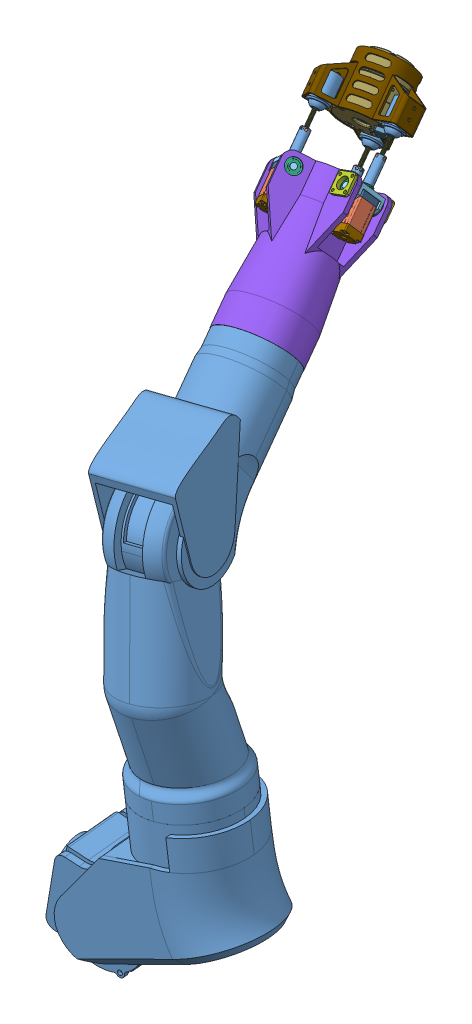
SolidWorks assembly 渲染用胳膊, configuration 默认. Lengths in mm.
Overall size (269.63 745.23 465.89).
177 component instances, 62 part files, 2 mates.
Components (placement in the parent):
- 左臂1-1: 左臂1 [默认] at (-529.8701 -324.4929 522.6027) size (209.74 530.01 223.26)
- 机械臂总装-1: 机械臂总装 [默认] at (59.2717 406.9847 293.0441) x (0.966024 0.189112 -0.176168) z (0.050994 0.528759 0.847239) size (122.17 276.98 210.32)
  - CRA-RI40-52-PRO-XX 2023.5.4 - Drum-1: CRA-RI40-52-PRO-XX 2023.5.4 - Drum [默认] at (-65.3352 0.778 -52.4868) x (-0.773511 0.267701 0.574471) z (-0.632199 -0.261859 -0.729215) size (67.95 60.31 67.96)
    - CRA-RI40-52-PRO-XX 2023.5.4 - Drum.stp-1: CRA-RI40-52-PRO-XX 2023.5.4 - Drum.stp [默认] at origin size (67.95 60.31 67.96)
      - CRA-RI40-52-PRO-XX_1_ASM.stp-1: CRA-RI40-52-PRO-XX_1_ASM.stp [默认] at origin size (67.95 60.31 67.96)
        - XB11-52__10001_ASM.stp-1: XB11-52__10001_ASM.stp [默认] at (0 16.8 0) x (0.703875 0 -0.710324) z (-0.710324 0 -0.703875) size (66.32 0.8 66.32)
          - XB11-52-06__10001.stp-1: XB11-52-06__10001.stp [默认] at (0 15.8 0) x (0.791272 0 -0.611464) z (-0.611464 0 -0.791272) size (47.28 0.81 47.28)
        - TINYMBS20WITHCONNECTOR2_ASM.stp-1: TINYMBS20WITHCONNECTOR2_ASM.stp [默认] at (2.7275 -27.9719 -6.5848) x (0 -1 0) z (0.92388 0 0.382683) size (0.82 3.25 5.53)
          - FH34SRJ8S05SH_STEP_STEP_ASM.stp-1: FH34SRJ8S05SH_STEP_STEP_ASM.stp [默认] at (-6.4719 -22.2833 0) x (0 0 -1) z (1 0 0) size (5.53 3.25 0.82)
            - NONE-51348.stp-1: NONE-51348.stp [默认] at origin size (0.15 0.3 0.08)
            - NONE-53783.stp-1: NONE-53783.stp [默认] at origin size (0.15 0.3 0.08)
            - NONE-55744.stp-1: NONE-55744.stp [默认] at origin size (0.15 0.08 0.08)
            - NONE-57763.stp-1: NONE-57763.stp [默认] at origin size (0.15 0.08 0.08)
            - NONE-60582.stp-1: NONE-60582.stp [默认] at origin size (0.15 0.3 0.08)
            - NONE-60979.stp-1: NONE-60979.stp [默认] at origin size (0.15 0.3 0.08)
            - NONE-62950.stp-1: NONE-62950.stp [默认] at origin size (0.15 0.3 0.08)
            - NONE-64179.stp-1: NONE-64179.stp [默认] at origin size (0.15 0.3 0.08)
            - NONE-65774.stp-1: NONE-65774.stp [默认] at origin size (0.15 0.08 0.08)
            - NONE-66548.stp-1: NONE-66548.stp [默认] at origin size (0.15 0.35 0.23)
            - NONE-67775.stp-1: NONE-67775.stp [默认] at origin size (0.15 0.35 0.23)
            - NONE-133224.stp-1: NONE-133224.stp [默认] at origin size (0.15 0.08 0.08)
            - NONE-134873.stp-1: NONE-134873.stp [默认] at origin size (0.15 0.3 0.08)
            - NONE-136443.stp-1: NONE-136443.stp [默认] at origin size (0.15 0.08 0.08)
            - NONE-141250.stp-1: NONE-141250.stp [默认] at origin size (0.15 0.35 0.23)
            - NONE-145287.stp-1: NONE-145287.stp [默认] at origin size (0.15 0.08 0.08)
            - NONE-147294.stp-1: NONE-147294.stp [默认] at origin size (0.15 0.08 0.08)
            - NONE-214429.stp-1: NONE-214429.stp [默认] at origin size (0.15 0.9 0.82)
            - NONE-214822.stp-1: NONE-214822.stp [默认] at origin size (0.15 0.3 0.08)
            - NONE-215190.stp-1: NONE-215190.stp [默认] at origin size (0.15 0.08 0.08)
            - NONE-216041.stp-1: NONE-216041.stp [默认] at origin size (0.15 0.35 0.23)
            - NONE-217624.stp-1: NONE-217624.stp [默认] at origin size (0.15 0.35 0.23)
            - NONE-222885.stp-1: NONE-222885.stp [默认] at origin size (0.15 0.35 0.23)
            - NONE-224875.stp-1: NONE-224875.stp [默认] at origin size (0.15 0.35 0.23)
            - NONE-228113.stp-1: NONE-228113.stp [默认] at origin size (0.15 0.9 0.82)
            - NONE-228916.stp-1: NONE-228916.stp [默认] at origin size (0.15 0.35 0.23)
        - CROSS_RECESSED_COUNTERSUNK_HE_1.stp-1: CROSS_RECESSED_COUNTERSUNK_HE_1.stp [默认] at (-21.8123 -33.1 2.8703) x (0 1 0) z (0.6 0 0.8) size (4 3.5 3.5)
        - RI40-52-D12-02__1000.stp-1: RI40-52-D12-02__1000.stp [默认] at (0 -15 0) x (0.382683 0 -0.92388) z (0.92388 0 0.382683) size (52.01 56.6 52)
        - CROSS_RECESSED_CHEESE_HEAD_SC_1.stp-1: CROSS_RECESSED_CHEESE_HEAD_SC_1.stp [默认] at (3.9505 15.5 -22.4044) x (0 -1 0) z (1 0 0) size (5.7 2.98 2.98)
        - MC50-D25X12_5_000.stp-1: MC50-D25X12_5_000.stp [默认] at (0.0001 -26.6014 0.0001) x (0.382686 0 -0.923879) z (0 -1 0) size (48.11 50.01 13.43)
        - CROSS_RECESSED_CHEESE_HEAD_SC_1.stp-2: CROSS_RECESSED_CHEESE_HEAD_SC_1.stp [默认] at (-3.9505 15.5 22.4044) x (0 -1 0) z (-1 0 0) size (5.7 2.98 2.98)
        - CROSS_RECESSED_COUNTERSUNK_HE_1.stp-2: CROSS_RECESSED_COUNTERSUNK_HE_1.stp [默认] at (-3.0048 -33.1 22.5417) x (0 1 0) z (0.395734 0 0.918365) size (4 3.5 3.5)
        - CROSS_RECESSED_CHEESE_HEAD_SC_1.stp-3: CROSS_RECESSED_CHEESE_HEAD_SC_1.stp [默认] at (-18.6357 15.5 13.0489) x (0 -1 0) z (-0.707107 0 -0.707107) size (5.7 2.98 2.98)
        - CROSS_RECESSED_COUNTERSUNK_HE_1.stp-3: CROSS_RECESSED_COUNTERSUNK_HE_1.stp [默认] at (18.8645 -33.1 -12.4259) x (0 1 0) z (0.188455 0 0.982082) size (4 3.5 3.5)
        - _M2X3_M2X3_100.stp-1: _M2X3_M2X3_100.stp [默认] at (-21.8118 -29.6014 2.8705) x (0.8 0 -0.6) z (0.6 0 0.8) size (3.23 5.8 2.8)
        - _M2X3_M2X3_100.stp-2: _M2X3_M2X3_100.stp [默认] at (-13.393 -29.6014 -17.4539) x (0.918365 0 -0.395734) z (0.395734 0 0.918365) size (3.23 5.8 2.8)
        - CROSS_RECESSED_CHEESE_HEAD_SC_1.stp-4: CROSS_RECESSED_CHEESE_HEAD_SC_1.stp [默认] at (-22.4044 15.5 -3.9505) x (0 -1 0) z (0 0 -1) size (5.7 2.98 2.98)
        - CROSS_RECESSED_CHEESE_HEAD_SC_1.stp-5: CROSS_RECESSED_CHEESE_HEAD_SC_1.stp [默认] at (13.0489 15.5 18.6357) x (0 -1 0) z (-0.707107 0 0.707107) size (5.7 2.98 2.98)
        - HEXAGON_SOCKET_HEAD_CAP_SCREW_1.stp-1: HEXAGON_SOCKET_HEAD_CAP_SCREW_1.stp [默认] at (19.8197 15.9 12.6265) x (0 -1 0) z (-0.954517 0 0.298155) size (22.5 4.5 4.5)
        - M2-3_10001.stp-1: M2-3_10001.stp [默认] at (0.7742 21 -17.7331) x (0.020141 0 0.999797) z (-0.999797 0 0.020141) size (4 5.4 4)
        - HEXAGON_SOCKET_HEAD_CAP_SCREW_1.stp-2: HEXAGON_SOCKET_HEAD_CAP_SCREW_1.stp [默认] at (-19.8197 15.9 -12.6265) x (0 -1 0) z (0.954517 0 -0.298155) size (22.5 4.5 4.5)
        - CROSS_RECESSED_CHEESE_HEAD_SC_1.stp-6: CROSS_RECESSED_CHEESE_HEAD_SC_1.stp [默认] at (18.6357 15.5 -13.0489) x (0 -1 0) z (0.707107 0 0.707107) size (5.7 2.98 2.98)
        - M2-3_10001.stp-2: M2-3_10001.stp [默认] at (-17.7331 21 -0.7742) x (0.999797 0 -0.020141) z (0.020141 0 0.999797) size (4 5.4 4)
        - _M2X3_M2X3_100.stp-3: _M2X3_M2X3_100.stp [默认] at (-3.0038 -29.6014 22.5414) x (0.982082 0 -0.188455) z (0.188455 0 0.982082) size (3.23 5.8 2.8)
        - M2-3_10001.stp-3: M2-3_10001.stp [默认] at (-0.7742 21 17.7331) x (-0.020141 0 -0.999797) z (0.999797 0 -0.020141) size (4 5.4 4)
        - _M2X3_M2X3_100.stp-4: _M2X3_M2X3_100.stp [默认] at (18.8646 -29.6014 -12.4267) size (3.23 5.8 2.8)
        - CROSS_RECESSED_COUNTERSUNK_HE_1.stp-4: CROSS_RECESSED_COUNTERSUNK_HE_1.stp [默认] at (-13.393 -33.1 -17.4539) x (0 1 0) z (0 0 1) size (4 3.5 3.5)
        - M2-3_10001.stp-4: M2-3_10001.stp [默认] at (17.7331 21 0.7742) x (-0.999797 0 0.020141) z (-0.020141 0 -0.999797) size (4 5.4 4)
        - CROSS_RECESSED_CHEESE_HEAD_SC_1.stp-7: CROSS_RECESSED_CHEESE_HEAD_SC_1.stp [默认] at (22.4044 15.5 3.9505) x (0 -1 0) z (0 0 1) size (5.7 2.98 2.98)
        - CROSS_RECESSED_CHEESE_HEAD_SC_1.stp-8: CROSS_RECESSED_CHEESE_HEAD_SC_1.stp [默认] at (-13.0489 15.5 -18.6357) x (0 -1 0) z (0.707107 0 -0.707107) size (5.7 2.98 2.98)
  - 手腕电机座-1: 手腕电机座 [默认] at (-66.8577 -30.748 -39.8459) x (-0.288066 -0.344371 -0.893547) z (0.956563 -0.147114 -0.251684) size (84.79 53 96.67)
  - 球铰2-1: 球铰2 [默认] at (-91.8577 2.9201 -23.4423) x (-0.727754 -0.224677 -0.647992) z (-0.684375 0.29959 0.664738) size (21 30.5 20.4)
  - 球铰2-2: 球铰2 [默认] at (-28.733 -6.7882 -40.0512) x (-0.228809 0.371791 0.899677) z (0.972441 0.044781 0.228809) size (21 30.5 20.4)
  - 球铰2-3: 球铰2 [默认] at (-76.7583 -21.6149 -82.813) x (0.956563 -0.147114 -0.251684) z (-0.288066 -0.344371 -0.893547) size (21 30.5 20.4)
  - 20NC38..31-1: 20NC38..31 [默认] at (-34.2487 -117.8316 4.4347) x (0.046372 0.927308 -0.371416) z (0.972366 0.043263 0.229417) size (109.8 25.88 45.74)
    - 20NC38..31.STEP-1: 20NC38..31.STEP [默认] at origin size (109.8 25.88 45.74)
      - 02-20-38.15________.STEP-1: 02-20-38.15________.STEP [默认] at origin size (39.65 25.88 45.74)
        - 02-20-38.STEP-1: 02-20-38.STEP [默认] at (20.075 0 0) x (0 0 1) z (-1 0 0) size (26.04 25.88 31.46)
          - 02-20-24.15_10-20-001-2.STEP-1: 02-20-24.15_10-20-001-2.STEP [默认] at origin size (20 20 24.15)
          - 13-20-8.5____.STEP-1: 13-20-8.5____.STEP [默认] at (0 0 16.075) x (0 1 0) z (0 0 -1) size (18.2 22.2 10.51)
          - 13-20-12.5______.STEP-1: 13-20-12.5______.STEP [默认] at (0 0 -14.575) x (0.707107 0.707107 0) z (0 0 1) size (18.3 18.3 15.8)
        - 03-20-008______38_______default.STEP-1: 03-20-008______38_______default.STEP [默认] at (3.8 0 0) x (1 0 0) z (0 0.78069 0.624918) size (32.3 16.26 16.27)
          - 06-20-008______38_________01-20-007-1.STEP-1: 06-20-008______38_________01-20-007-1.STEP [默认] at origin size (32.3 7 7)
          - 03-20-4.2-6YK_10-20-006-2.STEP-1: 03-20-4.2-6YK_10-20-006-2.STEP [默认] at (24.2 0 0) x (0 0.91534 0.402682) z (-1 0 0) size (12.06 12.08 4.2)
          - 10-20-001__________.STEP-1: 10-20-001__________.STEP [默认] at (16.9 0 0) x (0 0 1) z (-1 0 0) size (11.2 11.2 1.3)
          - 08-20-001______1_______07-20-001-1.STEP-1: 08-20-001______1_______07-20-001-1.STEP [默认] at (22.1 0 0) x (0 0 1) z (-1 0 0) size (11 11 1)
          - 08-20-001______1_______07-20-001-1.STEP-2: 08-20-001______1_______07-20-001-1.STEP [默认] at (11.4 0 0) x (0 0 1) z (-1 0 0) size (11 11 1)
          - 03-20-4.2-6YK_10-20-006-2.STEP-2: 03-20-4.2-6YK_10-20-006-2.STEP [默认] at (19 0 0) x (0 0.888249 0.459362) z (-1 0 0) size (12.06 12.08 4.2)
          - 03-20-4.2-6YK_10-20-006-2.STEP-3: 03-20-4.2-6YK_10-20-006-2.STEP [默认] at (13.5 0 0) x (0 0.91534 0.402682) z (-1 0 0) size (12.06 12.08 4.2)
          - 03-20-4.2-6YK_10-20-006-2.STEP-4: 03-20-4.2-6YK_10-20-006-2.STEP [默认] at (8.3 0 0) x (0 0.888249 0.459362) z (-1 0 0) size (12.06 12.08 4.2)
        - 01-20-003__20__________________.STEP-1: 01-20-003__20__________________.STEP [默认] at origin size (8.8 20 20)
        - 01-20-001__20__________________.STEP-1: 01-20-001__20__________________.STEP [默认] at (31.35 0 0) x (0 0 1) z (1 0 0) size (20 20 8.3)
        - 09-20-001____9X__5X4)_09-20-001.STEP-1: 09-20-001____9X__5X4)_09-20-001.STEP [默认] at (33.1 0 0) x (1 0 0) z (0 0.994502 0.104719) size (3 9 9)
        - 09-20-001____9X__5X4)_09-20-001.STEP-2: 09-20-001____9X__5X4)_09-20-001.STEP [默认] at (3.8 0 0) x (1 0 0) z (0 -0.49427 -0.869308) size (3 9 9)
        - 11-20-002__M2-37__20-42__.STEP-1: 11-20-002__M2-37__20-42__.STEP [默认] at (0.39 -7.7 7.7) x (0 0 -1) z (1 0 0) size (3 3 33)
        - 11-20-002__M2-37__20-42__.STEP-2: 11-20-002__M2-37__20-42__.STEP [默认] at (0.39 -7.7 -7.7) x (0 1 0) z (1 0 0) size (3 3 33)
        - 11-20-002__M2-37__20-42__.STEP-3: 11-20-002__M2-37__20-42__.STEP [默认] at (0.39 7.7 -7.7) x (0 0 1) z (1 0 0) size (3 3 33)
        - 11-20-002__M2-37__20-42__.STEP-4: 11-20-002__M2-37__20-42__.STEP [默认] at (0.39 7.7 7.7) x (0 -1 0) z (1 0 0) size (3 3 33)
        - 06-20-099__20___________20____________YK.STEP-1: 06-20-099__20___________20____________YK.STEP [默认] at (31.1 0 0) x (0 -0.624918 0.78069) z (-1 0 0) size (6.01 6.01 10)
        - 14-20-001__20-28____________________.STEP-1: 14-20-001__20-28____________________.STEP [默认] at (6.15 0 -8.6) x (0 -1 0) z (0 0 1) size (10.5 3.4 24.5)
      - 07-20-007__________________.STEP-1: 07-20-007__________________.STEP [默认] at (39.65 0 0) x (-1 0 0) z (0 -0.999857 -0.016895) size (6 12.92 13)
      - 07-20-013-2______________.STEP-1: 07-20-013-2______________.STEP [默认] at (68.4 0 0) x (0 -0.714016 0.700129) z (1 0 0) size (3.42 3.5 41.4)
      - 07-20-013-3______________.STEP-1: 07-20-013-3______________.STEP [默认] at (20.15 0 0) x (0 0.924225 0.381849) z (1 0 0) size (8 8 56.63)
      - 07-20-006__20______.STEP-1: 07-20-006__20______.STEP [默认] at (67.9 0 0) x (0 0.924225 0.381849) z (1 0 0) size (4.8 4.8 0.5)
      - 07-20-013-1__20_____________08-20-002-1.STEP-1: 07-20-013-1__20_____________08-20-002-1.STEP [默认] at (36.1 0 0) x (0 0.004204 -0.999991) z (1 0 0) size (9.01 9.01 35.91)
      - 07-20-002__20________________.STEP-1: 07-20-002__20________________.STEP [默认] at (69.65 0 0) x (0 0.004204 -0.999991) z (1 0 0) size (9.01 9.01 3.1)
  - 螺纹转换套-1: 螺纹转换套 [默认] at (-30.0844 -34.5593 -28.9185) x (-0.195243 -0.356231 -0.913772) z (0.046372 0.927308 -0.371416) size (5 5 5)
  - 球-1: 球 [默认] at (-29.7853 -28.5782 -31.3141) x (-0.55453 -0.285367 -0.781705) z (0.830871 -0.242211 -0.500987) size (14 13.45 14)
  - 球-2: 球 [默认] at (-92.91 -18.87 -14.7052) x (0.833324 -0.238487 -0.498693) z (0.551058 0.287142 0.783508) size (14 13.45 14)
  - 螺纹转换套-2: 螺纹转换套 [默认] at (-78.0965 -49.3819 -71.6684) x (0.952783 0.073148 0.29471) z (0.044309 0.926671 -0.373253) size (5 5 5)
  - 螺纹转换套-3: 螺纹转换套 [默认] at (-93.1916 -24.8538 -12.3142) x (-0.196131 -0.355877 -0.91372) z (0.043661 0.927725 -0.370703) size (5 5 5)
  - 球-3: 球 [默认] at (-77.8107 -43.4049 -74.0759) x (0.898492 0.126374 0.420407) z (-0.436749 0.353993 0.827006) size (14 13.45 14)
  - 20NC38..31-2: 20NC38..31 [默认] at (-82.0754 -132.597 -38.1503) x (0.044309 0.926671 -0.373253) z (-0.288139 -0.345888 -0.892937) size (109.8 25.88 45.74)
    - 20NC38..31.STEP-1: 20NC38..31.STEP [默认] at origin size (109.8 25.88 45.74)
      - 02-20-38.15________.STEP-1: 02-20-38.15________.STEP [默认] at origin size (39.65 25.88 45.74)
        - 02-20-38.STEP-1: 02-20-38.STEP [默认] at (20.075 0 0) x (0 0 1) z (-1 0 0) size (26.04 25.88 31.46)
          - 02-20-24.15_10-20-001-2.STEP-1: 02-20-24.15_10-20-001-2.STEP [默认] at origin size (20 20 24.15)
          - 13-20-8.5____.STEP-1: 13-20-8.5____.STEP [默认] at (0 0 16.075) x (0 1 0) z (0 0 -1) size (18.2 22.2 10.51)
          - 13-20-12.5______.STEP-1: 13-20-12.5______.STEP [默认] at (0 0 -14.575) x (0.707107 0.707107 0) z (0 0 1) size (18.3 18.3 15.8)
        - 03-20-008______38_______default.STEP-1: 03-20-008______38_______default.STEP [默认] at (3.8 0 0) x (1 0 0) z (0 0.78069 0.624918) size (32.3 16.26 16.27)
          - 06-20-008______38_________01-20-007-1.STEP-1: 06-20-008______38_________01-20-007-1.STEP [默认] at origin size (32.3 7 7)
          - 03-20-4.2-6YK_10-20-006-2.STEP-1: 03-20-4.2-6YK_10-20-006-2.STEP [默认] at (24.2 0 0) x (0 0.91534 0.402682) z (-1 0 0) size (12.06 12.08 4.2)
          - 10-20-001__________.STEP-1: 10-20-001__________.STEP [默认] at (16.9 0 0) x (0 0 1) z (-1 0 0) size (11.2 11.2 1.3)
          - 08-20-001______1_______07-20-001-1.STEP-1: 08-20-001______1_______07-20-001-1.STEP [默认] at (22.1 0 0) x (0 0 1) z (-1 0 0) size (11 11 1)
          - 08-20-001______1_______07-20-001-1.STEP-2: 08-20-001______1_______07-20-001-1.STEP [默认] at (11.4 0 0) x (0 0 1) z (-1 0 0) size (11 11 1)
          - 03-20-4.2-6YK_10-20-006-2.STEP-2: 03-20-4.2-6YK_10-20-006-2.STEP [默认] at (19 0 0) x (0 0.888249 0.459362) z (-1 0 0) size (12.06 12.08 4.2)
          - 03-20-4.2-6YK_10-20-006-2.STEP-3: 03-20-4.2-6YK_10-20-006-2.STEP [默认] at (13.5 0 0) x (0 0.91534 0.402682) z (-1 0 0) size (12.06 12.08 4.2)
          - 03-20-4.2-6YK_10-20-006-2.STEP-4: 03-20-4.2-6YK_10-20-006-2.STEP [默认] at (8.3 0 0) x (0 0.888249 0.459362) z (-1 0 0) size (12.06 12.08 4.2)
        - 01-20-003__20__________________.STEP-1: 01-20-003__20__________________.STEP [默认] at origin size (8.8 20 20)
        - 01-20-001__20__________________.STEP-1: 01-20-001__20__________________.STEP [默认] at (31.35 0 0) x (0 0 1) z (1 0 0) size (20 20 8.3)
        - 09-20-001____9X__5X4)_09-20-001.STEP-1: 09-20-001____9X__5X4)_09-20-001.STEP [默认] at (33.1 0 0) x (1 0 0) z (0 0.994502 0.104719) size (3 9 9)
        - 09-20-001____9X__5X4)_09-20-001.STEP-2: 09-20-001____9X__5X4)_09-20-001.STEP [默认] at (3.8 0 0) x (1 0 0) z (0 -0.49427 -0.869308) size (3 9 9)
        - 11-20-002__M2-37__20-42__.STEP-1: 11-20-002__M2-37__20-42__.STEP [默认] at (0.39 -7.7 7.7) x (0 0 -1) z (1 0 0) size (3 3 33)
        - 11-20-002__M2-37__20-42__.STEP-2: 11-20-002__M2-37__20-42__.STEP [默认] at (0.39 -7.7 -7.7) x (0 1 0) z (1 0 0) size (3 3 33)
        - 11-20-002__M2-37__20-42__.STEP-3: 11-20-002__M2-37__20-42__.STEP [默认] at (0.39 7.7 -7.7) x (0 0 1) z (1 0 0) size (3 3 33)
        - 11-20-002__M2-37__20-42__.STEP-4: 11-20-002__M2-37__20-42__.STEP [默认] at (0.39 7.7 7.7) x (0 -1 0) z (1 0 0) size (3 3 33)
        - 06-20-099__20___________20____________YK.STEP-1: 06-20-099__20___________20____________YK.STEP [默认] at (31.1 0 0) x (0 -0.624918 0.78069) z (-1 0 0) size (6.01 6.01 10)
        - 14-20-001__20-28____________________.STEP-1: 14-20-001__20-28____________________.STEP [默认] at (6.15 0 -8.6) x (0 -1 0) z (0 0 1) size (10.5 3.4 24.5)
      - 07-20-007__________________.STEP-1: 07-20-007__________________.STEP [默认] at (39.65 0 0) x (-1 0 0) z (0 -0.999857 -0.016895) size (6 12.92 13)
      - 07-20-013-2______________.STEP-1: 07-20-013-2______________.STEP [默认] at (68.4 0 0) x (0 -0.714016 0.700129) z (1 0 0) size (3.42 3.5 41.4)
      - 07-20-013-3______________.STEP-1: 07-20-013-3______________.STEP [默认] at (20.15 0 0) x (0 0.924225 0.381849) z (1 0 0) size (8 8 56.63)
      - 07-20-006__20______.STEP-1: 07-20-006__20______.STEP [默认] at (67.9 0 0) x (0 0.924225 0.381849) z (1 0 0) size (4.8 4.8 0.5)
      - 07-20-013-1__20_____________08-20-002-1.STEP-1: 07-20-013-1__20_____________08-20-002-1.STEP [默认] at (36.1 0 0) x (0 0.004204 -0.999991) z (1 0 0) size (9.01 9.01 35.91)
      - 07-20-002__20________________.STEP-1: 07-20-002__20________________.STEP [默认] at (69.65 0 0) x (0 0.004204 -0.999991) z (1 0 0) size (9.01 9.01 3.1)
  - 20NC38..31-3: 20NC38..31 [默认] at (-97.1124 -108.1635 20.9749) x (0.043661 0.927725 -0.370703) z (-0.684447 0.298072 0.665346) size (109.8 25.88 45.74)
    - 20NC38..31.STEP-1: 20NC38..31.STEP [默认] at origin size (109.8 25.88 45.74)
      - 02-20-38.15________.STEP-1: 02-20-38.15________.STEP [默认] at origin size (39.65 25.88 45.74)
        - 02-20-38.STEP-1: 02-20-38.STEP [默认] at (20.075 0 0) x (0 0 1) z (-1 0 0) size (26.04 25.88 31.46)
          - 02-20-24.15_10-20-001-2.STEP-1: 02-20-24.15_10-20-001-2.STEP [默认] at origin size (20 20 24.15)
          - 13-20-8.5____.STEP-1: 13-20-8.5____.STEP [默认] at (0 0 16.075) x (0 1 0) z (0 0 -1) size (18.2 22.2 10.51)
          - 13-20-12.5______.STEP-1: 13-20-12.5______.STEP [默认] at (0 0 -14.575) x (0.707107 0.707107 0) z (0 0 1) size (18.3 18.3 15.8)
        - 03-20-008______38_______default.STEP-1: 03-20-008______38_______default.STEP [默认] at (3.8 0 0) x (1 0 0) z (0 0.78069 0.624918) size (32.3 16.26 16.27)
          - 06-20-008______38_________01-20-007-1.STEP-1: 06-20-008______38_________01-20-007-1.STEP [默认] at origin size (32.3 7 7)
          - 03-20-4.2-6YK_10-20-006-2.STEP-1: 03-20-4.2-6YK_10-20-006-2.STEP [默认] at (24.2 0 0) x (0 0.91534 0.402682) z (-1 0 0) size (12.06 12.08 4.2)
          - 10-20-001__________.STEP-1: 10-20-001__________.STEP [默认] at (16.9 0 0) x (0 0 1) z (-1 0 0) size (11.2 11.2 1.3)
          - 08-20-001______1_______07-20-001-1.STEP-1: 08-20-001______1_______07-20-001-1.STEP [默认] at (22.1 0 0) x (0 0 1) z (-1 0 0) size (11 11 1)
          - 08-20-001______1_______07-20-001-1.STEP-2: 08-20-001______1_______07-20-001-1.STEP [默认] at (11.4 0 0) x (0 0 1) z (-1 0 0) size (11 11 1)
          - 03-20-4.2-6YK_10-20-006-2.STEP-2: 03-20-4.2-6YK_10-20-006-2.STEP [默认] at (19 0 0) x (0 0.888249 0.459362) z (-1 0 0) size (12.06 12.08 4.2)
          - 03-20-4.2-6YK_10-20-006-2.STEP-3: 03-20-4.2-6YK_10-20-006-2.STEP [默认] at (13.5 0 0) x (0 0.91534 0.402682) z (-1 0 0) size (12.06 12.08 4.2)
          - 03-20-4.2-6YK_10-20-006-2.STEP-4: 03-20-4.2-6YK_10-20-006-2.STEP [默认] at (8.3 0 0) x (0 0.888249 0.459362) z (-1 0 0) size (12.06 12.08 4.2)
        - 01-20-003__20__________________.STEP-1: 01-20-003__20__________________.STEP [默认] at origin size (8.8 20 20)
        - 01-20-001__20__________________.STEP-1: 01-20-001__20__________________.STEP [默认] at (31.35 0 0) x (0 0 1) z (1 0 0) size (20 20 8.3)
        - 09-20-001____9X__5X4)_09-20-001.STEP-1: 09-20-001____9X__5X4)_09-20-001.STEP [默认] at (33.1 0 0) x (1 0 0) z (0 0.994502 0.104719) size (3 9 9)
        - 09-20-001____9X__5X4)_09-20-001.STEP-2: 09-20-001____9X__5X4)_09-20-001.STEP [默认] at (3.8 0 0) x (1 0 0) z (0 -0.49427 -0.869308) size (3 9 9)
        - 11-20-002__M2-37__20-42__.STEP-1: 11-20-002__M2-37__20-42__.STEP [默认] at (0.39 -7.7 7.7) x (0 0 -1) z (1 0 0) size (3 3 33)
        - 11-20-002__M2-37__20-42__.STEP-2: 11-20-002__M2-37__20-42__.STEP [默认] at (0.39 -7.7 -7.7) x (0 1 0) z (1 0 0) size (3 3 33)
        - 11-20-002__M2-37__20-42__.STEP-3: 11-20-002__M2-37__20-42__.STEP [默认] at (0.39 7.7 -7.7) x (0 0 1) z (1 0 0) size (3 3 33)
        - 11-20-002__M2-37__20-42__.STEP-4: 11-20-002__M2-37__20-42__.STEP [默认] at (0.39 7.7 7.7) x (0 -1 0) z (1 0 0) size (3 3 33)
        - 06-20-099__20___________20____________YK.STEP-1: 06-20-099__20___________20____________YK.STEP [默认] at (31.1 0 0) x (0 -0.624918 0.78069) z (-1 0 0) size (6.01 6.01 10)
        - 14-20-001__20-28____________________.STEP-1: 14-20-001__20-28____________________.STEP [默认] at (6.15 0 -8.6) x (0 -1 0) z (0 0 1) size (10.5 3.4 24.5)
      - 07-20-007__________________.STEP-1: 07-20-007__________________.STEP [默认] at (39.65 0 0) x (-1 0 0) z (0 -0.999857 -0.016895) size (6 12.92 13)
      - 07-20-013-2______________.STEP-1: 07-20-013-2______________.STEP [默认] at (68.4 0 0) x (0 -0.714016 0.700129) z (1 0 0) size (3.42 3.5 41.4)
      - 07-20-013-3______________.STEP-1: 07-20-013-3______________.STEP [默认] at (20.15 0 0) x (0 0.924225 0.381849) z (1 0 0) size (8 8 56.63)
      - 07-20-006__20______.STEP-1: 07-20-006__20______.STEP [默认] at (67.9 0 0) x (0 0.924225 0.381849) z (1 0 0) size (4.8 4.8 0.5)
      - 07-20-013-1__20_____________08-20-002-1.STEP-1: 07-20-013-1__20_____________08-20-002-1.STEP [默认] at (36.1 0 0) x (0 0.004204 -0.999991) z (1 0 0) size (9.01 9.01 35.91)
      - 07-20-002__20________________.STEP-1: 07-20-002__20________________.STEP [默认] at (69.65 0 0) x (0 0.004204 -0.999991) z (1 0 0) size (9.01 9.01 3.1)
  - 电缸座-1: 电缸座 [默认] at (-95.2721 -69.0599 5.3498) x (0.727754 0.224677 0.647992) z (-0.043661 -0.927725 0.370703) size (42 20 14)
  - F696.ZZ-1: F696.ZZ [默认] at (-84.6614 -72.1838 17.6646) x (0.148454 0.870814 -0.468663) z (0.669578 -0.437269 -0.600384) size (17 5 17)
  - F696.ZZ-2: F696.ZZ [默认] at (-106.494 -78.9241 -1.7752) x (-0.284553 0.958575 -0.012786) z (-0.624022 -0.175083 0.761539) size (17 5 17)
  - 轴承端盖-2: 轴承端盖 [默认] at (-38.1559 -76.2394 13.1516) x (-0.044781 -0.927236 0.371791) z (0.228809 -0.371791 -0.899677) size (20.14 20.14 5)
  - 轴承端盖-3: 轴承端盖 [默认] at (-27.0815 -94.234 -30.3928) x (-0.044781 -0.927236 0.371791) z (-0.228809 0.371791 0.899677) size (20.14 20.14 5)
  - 电缸座-4: 电缸座 [默认] at (-32.2941 -78.7455 -11.2205) x (0.228809 -0.371791 -0.899677) z (-0.046372 -0.927308 0.371416) size (42 20 14)
  - 电缸座-5: 电缸座 [默认] at (-80.2078 -93.5378 -53.8829) x (-0.956563 0.147114 0.251684) z (-0.044309 -0.926671 0.373253) size (42 20 14)
  - 手腕关节-1: 手腕关节 [默认] at (-75.7512 -214.8969 33.9919) x (0.972441 0.044781 0.228809) z (-0.228809 0.371791 0.899677) size (93.36 150 107.8)
  - F696.ZZ-7: F696.ZZ [默认] at (-29.1866 -90.8136 -22.1158) x (-0.103795 0.909608 -0.402293) z (-0.967922 -0.18543 -0.169536) size (17 5 17)
  - F696.ZZ-9: F696.ZZ [默认] at (-94.8664 -97.8178 -47.4949) x (-0.050847 0.765907 -0.640938) z (0.287058 0.625895 0.725158) size (17 5 17)
  - F696.ZZ-10: F696.ZZ [默认] at (-66.1695 -102.2312 -55.0454) x (-0.036507 0.796088 -0.604079) z (-0.289231 -0.587028 -0.756137) size (17 5 17)
  - F696.ZZ-11: F696.ZZ [默认] at (-36.0508 -79.6598 4.8745) x (-0.228512 0.877857 -0.42089) z (0.946271 0.30189 0.115903) size (17 5 17)
Mates (geometry in assembly coordinates):
- 重合1: coincident: plane of 左臂1-1 through (42.2768 232.8192 442.8838) normal (-0.210637 0.579109 -0.787569); plane of 机械臂总装-1/手腕关节-1 through (79.8657 246.4967 442.8878) normal (0.210637 -0.579109 0.787569)
- 同心1: concentric aligned: cylinder of 左臂1-1 through (42.2768 232.8192 442.8838) axis (-0.210637 0.579109 -0.787569) radius 39.7603; cylinder of 机械臂总装-1/手腕关节-1 through (6.9582 329.9216 310.8277) axis (-0.210637 0.579109 -0.787569) radius 40
